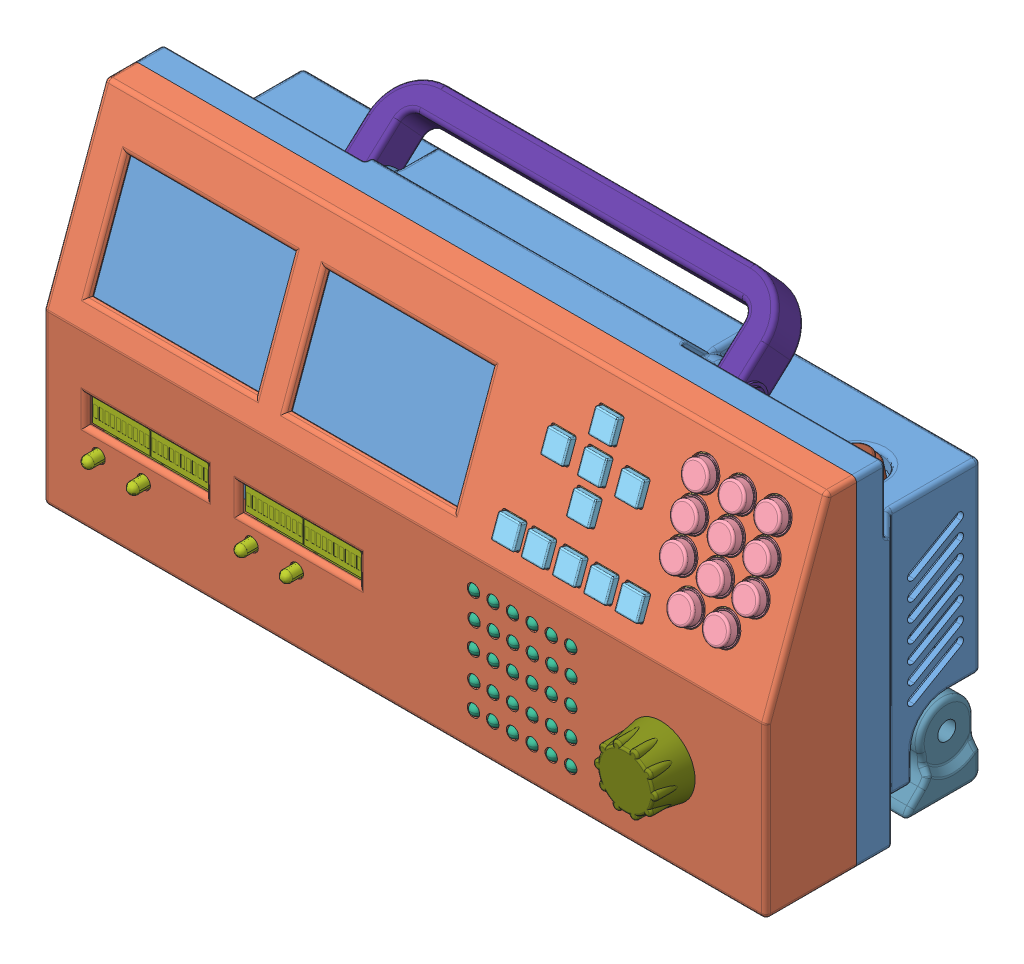
SolidWorks assembly Assembly, configuration Default. Lengths in mm.
Overall size (320 163.77 122.5).
42 component instances, 19 part files, 60 mates.
Components (placement in the parent):
- back_panel-1: back_panel [Default] at (2.4805 137.3007 327.5221) size (320 150.18 65)
- front_panel-1: front_panel [Default] at (322.4805 137.3007 342.5221) x (-1 0 0) z (0 0 -1) size (320 150.18 40)
- keypad_with_keycaps-1: keypad_with_keycaps [Default] at origin size (121.92 70.52 35.06)
  - Keypad-1: Keypad [Default] at (155.1031 162.0529 392.6379) x (1 0 0) z (0 0.34202 0.939693) size (121.92 71.12 10.8)
  - button_cap_round-1: button_cap_round [Default] at (304.9631 270.5 353.4325) x (-1 0 0) z (0 0.34202 0.939693) size (12.8 12.8 8.2)
  - button_cap_round-2: button_cap_round [Default] at (289.2151 270.5 353.4325) x (-1 0 0) z (0 0.34202 0.939693) size (12.8 12.8 8.2)
  - button_cap_round-3: button_cap_round [Default] at (272.9591 270.5 353.4325) x (-1 0 0) z (0 0.34202 0.939693) size (12.8 12.8 8.2)
  - button_cap_round-4: button_cap_round [Default] at (304.9631 257.1338 358.2973) x (-1 0 0) z (0 0.34202 0.939693) size (12.8 12.8 8.2)
  - button_cap_round-5: button_cap_round [Default] at (289.2151 257.1338 358.2973) x (-1 0 0) z (0 0.34202 0.939693) size (12.8 12.8 8.2)
  - button_cap_round-6: button_cap_round [Default] at (272.9591 257.1338 358.2973) x (-1 0 0) z (0 0.34202 0.939693) size (12.8 12.8 8.2)
  - button_cap_round-7: button_cap_round [Default] at (304.9631 243.7676 363.1622) x (-1 0 0) z (0 0.34202 0.939693) size (12.8 12.8 8.2)
  - button_cap_round-8: button_cap_round [Default] at (289.2151 243.7676 363.1622) x (-1 0 0) z (0 0.34202 0.939693) size (12.8 12.8 8.2)
  - button_cap_round-9: button_cap_round [Default] at (272.9591 243.7676 363.1622) x (-1 0 0) z (0 0.34202 0.939693) size (12.8 12.8 8.2)
  - button_cap_round-10: button_cap_round [Default] at (296.8351 230.4014 368.0271) x (-1 0 0) z (0 0.34202 0.939693) size (12.8 12.8 8.2)
  - button_cap_round-11: button_cap_round [Default] at (281.0871 230.4014 368.0271) x (-1 0 0) z (0 0.34202 0.939693) size (12.8 12.8 8.2)
  - button_cap_square-1: button_cap_square [Default] at (231.3031 255.2243 358.9923) x (1 0 0) z (0 0.34202 0.939693) size (10 10 6.2)
  - button_cap_square-2: button_cap_square [Default] at (231.3031 268.5905 354.1274) x (1 0 0) z (0 0.34202 0.939693) size (10 10 6.2)
  - button_cap_square-3: button_cap_square [Default] at (247.7131 255.2619 358.9787) x (1 0 0) z (0 0.34202 0.939693) size (10 10 6.2)
  - button_cap_square-4: button_cap_square [Default] at (215.0471 255.2243 358.9923) x (1 0 0) z (0 0.34202 0.939693) size (10 10 6.2)
  - button_cap_square-5: button_cap_square [Default] at (231.3031 241.9258 363.8326) x (1 0 0) z (0 0.34202 0.939693) size (10 10 6.2)
  - button_cap_square-6: button_cap_square [Default] at (204.8871 223.241 370.6333) x (1 0 0) z (0 0.34202 0.939693) size (10 10 6.2)
  - button_cap_square-7: button_cap_square [Default] at (218.0951 223.1216 370.6768) x (1 0 0) z (0 0.34202 0.939693) size (10 10 6.2)
  - button_cap_square-8: button_cap_square [Default] at (231.9381 223.1216 370.6768) x (1 0 0) z (0 0.34202 0.939693) size (10 10 6.2)
  - button_cap_square-9: button_cap_square [Default] at (245.7811 223.1216 370.6768) x (1 0 0) z (0 0.34202 0.939693) size (10 10 6.2)
  - button_cap_square-10: button_cap_square [Default] at (259.6241 223.1216 370.6768) x (1 0 0) z (0 0.34202 0.939693) size (10 10 6.2)
- LEDmatrix-1: LEDmatrix [Default] at (63.8045 79.9307 374.1221) size (64.13 65.66 10.01)
- LED_bars-1: LED_bars [Default] at (146.3805 197.4507 373.7106) x (0 -1 0) z (0 0 -1) size (39.75 57.75 38.1)
- LED_bars-2: LED_bars [Default] at (78.6305 197.4507 373.7106) x (0 -1 0) z (0 0 -1) size (39.75 57.75 38.1)
- potentiometer_B10K-1: potentiometer_B10K [Default] at (277.4318 177.2007 371.1221) x (0 -1 0) z (0 0 1) size (17 26.43 27.6)
- PSU-1: PSU [Default] at (165.6805 292.9007 291.6135) x (0 -1 0) z (0 0 1) size (46.8 37.5 15.1)
- MCU-2: MCU [Default] at (160.3185 237.8214 291.5693) x (-1 0 0) z (0 0 1) size (75.96 70.87 10.4)
- power switch-1: power switch [Default] at (287.4805 251.9761 307.5221) x (0.939025 0 0.34385) z (-0.34385 0 0.939025) size (19 38 19)
- DC_JACK-1: DC_JACK [Default] at (296.4805 202.3007 279.9221) x (0 1 0) z (0 0 -1) size (9.26 14.51 14.45)
- foot_right-1: foot_right [Default] at (27.4805 137.3007 327.5221) x (0 0 1) z (-1 0 0) size (32.66 35 18.16)
- foot_left-1: foot_left [Default] at (297.4805 137.3007 327.5221) x (0 0 1) z (-1 0 0) size (32.66 35 18.16)
- foot_chip-1: foot_chip [Default] at (25.0805 137.3007 342.5221) x (0 0 1) z (-1 0 0) size (23.38 5.24 35.8)
- foot_chip-2: foot_chip [Default] at (264.0805 137.3007 342.5221) x (0 0 1) z (-1 0 0) size (23.38 5.24 35.8)
- knob-1: knob [Default] at (277.4318 177.2007 383.9221) x (0 1 0) z (1 0 0) size (30 16.1 30)
- handle-1: handle [Default] at (162.4805 286.3387 299.3291) x (-1 0 0) z (0 0.673665 -0.739037) size (179 18 49)
- display_fastener_chip-1: display_fastener_chip [Default] at (102.4805 272.9078 350.6725) x (1 0 0) z (0 -0.939693 0.34202) size (35 1.6 17.5)
- LCD_display-1: LCD_display [Default] at (55.4805 244.1549 366.2457) x (1 0 0) z (0 -0.939693 0.34202) size (86 5 56)
- LCD_display-2: LCD_display [Default] at (143.4805 244.1549 366.2457) x (1 0 0) z (0 -0.939693 0.34202) size (86 5 56)
Mates (geometry in assembly coordinates):
- Coincident15: coincident aligned: plane of LED_bars-1 through (124.0204 187.2607 372.4121) normal (0 1 0); plane of LED_bars-2 through (56.2704 187.2607 372.4121) normal (0 1 0)
- Coincident16: coincident aligned: plane of LED_bars-1 through (124.0204 182.1807 380.4121) normal (0 0 1); plane of LED_bars-2 through (56.2704 182.1807 380.4121) normal (0 0 1)
- Distance3: distance = 6 mm anti-aligned: plane of front_panel-1 through (2.4805 137.3007 380.1221) normal (0 0 -1); plane of LEDmatrix-1 through (208.013 177.5302 374.1221) normal (0 0 1)
- Distance4: distance = 2 mm anti-aligned: plane of potentiometer_B10K-1 through (277.4318 177.2007 378.1221) normal (0 0 1); plane of front_panel-1 through (2.4805 137.3007 380.1221) normal (0 0 -1)
- Distance5: distance = 80 mm anti-aligned: plane of LEDmatrix-1 through (240.0805 144.7007 373.7106) normal (1 0 0); plane of front_panel-1 through (320.0805 137.3007 342.5221) normal (-1 0 0)
- Distance8: distance = 5 mm anti-aligned: plane of LEDmatrix-1 through (175.9455 144.7007 373.7106) normal (0 -1 0); plane of front_panel-1 through (2.4805 139.7007 342.5221) normal (0 1 0)
- Distance9: distance = 16 mm anti-aligned: plane of LED_bars-2 through (20.8805 197.4507 374.1221) normal (-1 0 0); plane of front_panel-1 through (4.8805 137.3007 342.5221) normal (1 0 0)
- Distance10: distance = 10 mm anti-aligned: plane of LED_bars-2 through (78.6305 157.7007 374.1221) normal (1 0 0); plane of LED_bars-1 through (88.6305 197.4507 374.1221) normal (-1 0 0)
- Distance11: distance = 6 mm anti-aligned: plane of LED_bars-2 through (49.7555 177.5757 374.1221) normal (0 0 1); plane of front_panel-1 through (2.4805 137.3007 380.1221) normal (0 0 -1)
- Distance13: distance = 18 mm anti-aligned: plane of front_panel-1 through (2.4805 139.7007 342.5221) normal (0 1 0); plane of LED_bars-1 through (88.6305 157.7007 374.1221) normal (0 -1 0)
- Coincident31: coincident aligned: plane of back_panel-1 through (322.4805 137.3007 342.5221) normal (1 0 0); plane of front_panel-1 through (322.4805 137.3007 342.5221) normal (1 0 0)
- Coincident32: coincident aligned: plane of back_panel-1 through (2.4805 287.4761 342.5221) normal (0 1 0); plane of front_panel-1 through (2.4805 287.4761 355.1605) normal (0 1 0)
- Coincident33: coincident anti-aligned: plane of back_panel-1 through (2.4805 137.3007 342.5221) normal (0 0 1); plane of front_panel-1 through (2.4805 287.4761 342.5221) normal (0 0 -1)
- Distance17: distance = 70 mm anti-aligned: plane of MCU-2 through (84.8805 168.2254 289.9221) normal (-1 0 0); plane of back_panel-1 through (14.8805 277.4761 277.5221) normal (1 0 0)
- Width2: width anti-aligned: plane of MCU-2 through (86.1505 237.8214 289.9221) normal (0 1 0); plane of back_panel-1 through (159.0485 166.9554 289.9221) normal (0 -1 0); plane of MCU-2 through (322.4805 255.0761 330.0221) normal (0 -1 0); plane of back_panel-1 through (312.4805 149.7007 277.5221) normal (0 1 0)
- Distance18: distance = 70 mm aligned: plane of PSU-1 through (240.0805 200.4307 289.9221) normal (-1 0 0); plane of back_panel-1 through (310.0805 277.4761 277.5221) normal (-1 0 0)
- Distance19: distance = 5.2 mm anti-aligned: plane of PSU-1 through (241.3505 154.9007 289.9221) normal (0 -1 0); plane of back_panel-1 through (312.4805 149.7007 277.5221) normal (0 1 0)
- Coincident37: coincident anti-aligned: plane of back_panel-1 through (88.2285 169.9054 289.9221) normal (0 0 1); plane of MCU-2 through (122.5995 202.3884 289.9221) normal (0 0 -1)
- Coincident38: coincident anti-aligned: plane of back_panel-1 through (243.1805 198.6507 289.9221) normal (0 0 1); plane of PSU-1 through (258.8305 178.3007 289.9221) normal (0 0 -1)
- Concentric2: concentric aligned: cylinder of back_panel-1 through (287.4805 230.1913 307.5221) axis (0 1 0) radius 6.5; cylinder of power switch-1 through (287.4805 223.9761 307.5221) axis (0 1 0) radius 5.25
- Distance14: distance = 1 mm anti-aligned: plane of power switch-1 through (287.4805 251.9761 307.5221) normal (0 -1 0); plane of back_panel-1 through (287.4805 250.9761 307.5221) normal (0 1 0)
- Parallel1: parallel aligned: plane of back_panel-1 through (310.0805 277.4761 277.5221) normal (-1 0 0); plane of DC_JACK-1 through (290.9805 206.5507 279.9221) normal (-1 0 0)
- Concentric4: concentric anti-aligned: circle of DC_JACK-1; cylinder of back_panel-1 through (297.4805 202.3007 298.3069) axis (0 0 -1) radius 6.5
- Coincident42: coincident anti-aligned: plane of back_panel-1 through (2.4805 137.3007 279.9221) normal (0 0 1); plane of DC_JACK-1 through (296.4805 202.3007 279.9221) normal (0 0 -1)
- Parallel2: parallel aligned: plane of front_panel-1 through (320.0805 137.3007 342.5221) normal (-1 0 0); plane of potentiometer_B10K-1 through (265.0805 184.7007 378.1221) normal (-1 0 0)
- Distance15: distance = 55 mm aligned: plane of potentiometer_B10K-1 through (265.0805 184.7007 378.1221) normal (-1 0 0); plane of front_panel-1 through (320.0805 137.3007 342.5221) normal (-1 0 0)
- Distance16: distance = 30 mm anti-aligned: plane of potentiometer_B10K-1 through (265.0805 169.7007 378.1221) normal (0 -1 0); plane of front_panel-1 through (2.4805 139.7007 342.5221) normal (0 1 0)
- InPlace1: in place: plane of back_panel-1 through (27.4805 160.3007 292.5221) normal (-1 0 0); plane of ? through (27.4805 0 0) normal (-1 0 0); moOrthogonalPlaneRef_w of back_panel-1 through (27.4805 160.3007 292.5221) normal (-1 0 0); plane of ? through (27.4805 0 0) normal (0 1 0); plane of back_panel-1 through (27.4805 160.3007 292.5221) normal (-1 0 0); plane of ? through (27.4805 0 0) normal (0 0 1); plane of back_panel-1 through (27.4805 160.3007 292.5221) normal (-1 0 0); unknown of foot_right-1
- Coincident43: coincident aligned: plane of back_panel-1; plane of foot_right-1
- Coincident44: coincident aligned: moOrthogonalPlaneRef_w of back_panel-1 through (27.4805 137.3007 327.5221) normal (0 1 0); plane of footer^Assembly-1 through (27.4805 137.3007 327.5221) normal (0 1 0)
- Coincident45: coincident anti-aligned: moOrthogonalPlaneRef_w of back_panel-1 through (27.4805 137.3007 327.5221) normal (0 0 -1); plane of footer^Assembly-1 through (27.4805 137.3007 327.5221) normal (0 0 1)
- Coincident43: coincident anti-aligned: plane of back_panel-1 through (297.4805 160.3007 292.5221) normal (1 0 0); plane of foot_left-1 through (297.4805 137.3007 307.0196) normal (-1 0 0)
- Concentric5: concentric aligned: circle of foot_right-1; circle of foot_left-1
- InPlace2: in place: plane of front_panel-1 through (25.0805 141.3007 342.5221) normal (-1 0 0); plane of ? through (25.0805 0 0) normal (-1 0 0); plane of front_panel-1 through (25.0805 141.3007 342.5221) normal (-1 0 0); plane of ? through (25.0805 0 0) normal (0 1 0); plane of front_panel-1 through (25.0805 141.3007 342.5221) normal (-1 0 0); plane of ? through (25.0805 0 0) normal (0 0 1); plane of front_panel-1 through (25.0805 141.3007 342.5221) normal (-1 0 0); unknown of foot_chip-1
- Coincident46: coincident aligned: plane of front_panel-1; plane of foot_chip-1
- Coincident47: coincident aligned: moOrthogonalPlaneRef_w of front_panel-1 through (25.0805 137.3007 342.5221) normal (0 1 0); plane of foot_chip-1 through (25.0805 137.3007 342.5221) normal (0 1 0)
- Coincident48: coincident anti-aligned: moOrthogonalPlaneRef_w of front_panel-1 through (25.0805 137.3007 342.5221) normal (0 0 -1); plane of foot_chip-1 through (25.0805 137.3007 342.5221) normal (0 0 1)
- Coincident49: coincident aligned: plane of front_panel-1 through (299.8805 141.3007 342.5221) normal (1 0 0); plane of foot_chip-2 through (299.8805 141.3007 342.5221) normal (1 0 0)
- Concentric6: concentric aligned: cylinder of front_panel-1 through (304.0524 141.3007 369.0221) axis (-1 0 0) radius 1.475; cylinder of foot_chip-2 through (303.3736 141.3007 369.0221) axis (-1 0 0) radius 1.235
- Coincident50: coincident aligned: plane of foot_right-1 through (9.4805 137.3007 280.5221) normal (0 -1 0); plane of foot_left-1 through (315.4805 137.3007 280.5221) normal (0 -1 0)
- Coincident51: coincident aligned: plane of foot_chip-1 through (1.3719 137.3007 346.5777) normal (0 -1 0); plane of foot_chip-2 through (240.3719 137.3007 346.5777) normal (0 -1 0)
- Concentric8: concentric anti-aligned: cylinder of potentiometer_B10K-1 through (277.4318 177.2007 387.7221) axis (0 0 -1) radius 3.5; cylinder of knob-1 through (277.4318 177.2007 371.477) axis (0 0 1) radius 4.4
- Coincident52: coincident anti-aligned: plane of potentiometer_B10K-1 through (277.4318 177.2007 398.7221) normal (0 0 1); plane of knob-1 through (277.4318 177.2007 398.7221) normal (0 0 -1)
- Width4: width aligned: plane of handle-1 through (85.9805 315.6476 280.5358) normal (1 0 0); plane of handle-1 through (238.9805 315.6476 280.5358) normal (-1 0 0); plane of back_panel-1 through (238.4805 267.4761 320.0221) normal (1 0 0); plane of back_panel-1 through (86.4805 267.4761 320.0221) normal (-1 0 0)
- Concentric11: concentric aligned: circle of back_panel-1; circle of handle-1
- Coincident53: coincident anti-aligned: plane of front_panel-1 through (322.4805 156.3304 394.8059) normal (0 -0.34202 -0.939693); plane of display_fastener_chip-1 through (102.4805 273.455 352.176) normal (0 0.34202 0.939693)
- Concentric12: concentric anti-aligned: circle of front_panel-1; circle of display_fastener_chip-1
- LimitAngle1: limit planar angle = 0.739157 rad aligned: plane of back_panel-1 through (322.4805 257.4761 330.0221) normal (0 1 0); plane of handle-1 through (85.9805 301.074 296.5236) normal (0 0.739037 0.673665)
- LimitAngle2: limit planar angle = 0 rad aligned: plane of front_panel-1 through (322.4805 137.3007 342.5221) normal (0 1 0); plane of knob-1 through (277.4318 177.2007 383.9221) normal (0 1 0)
- Concentric13: concentric aligned: circle of front_panel-1; cylinder of knob-1 through (277.4318 177.2007 371.077) axis (0 0 1) radius 2.8
- Distance20: distance = 1 mm anti-aligned: plane of knob-1 through (277.4318 177.2007 383.9221) normal (0 0 -1); plane of front_panel-1 through (2.4805 137.3007 382.5221) normal (0 0 1)
- Coincident124: coincident anti-aligned: plane of front_panel-1 through (2.4805 211.4798 380.2668) normal (0 -0.34202 -0.939693); plane of LCD_display-1 through (55.4805 244.8389 368.1251) normal (0 0.34202 0.939693)
- Width5: width aligned: plane of front_panel-1 through (17.4805 221.6976 379.1019) normal (0.866025 0.17101 0.469846); plane of front_panel-1 through (93.4805 221.6976 379.1019) normal (-0.866025 0.17101 0.469846); plane of LCD_display-1 through (18.4805 221.8164 376.5046) normal (-1 0 0); plane of LCD_display-1 through (92.4805 221.8164 376.5046) normal (1 0 0)
- Width6: width aligned: plane of front_panel-1 through (17.4805 269.6219 361.6589) normal (0 -0.642788 0.766044); plane of front_panel-1 through (17.4805 221.6976 379.1019) normal (0 0.984808 0.173648); plane of LCD_display-1 through (18.4805 267.8614 359.7456) normal (0 0.939693 -0.34202); plane of LCD_display-1 through (18.4805 221.8164 376.5046) normal (0 -0.939693 0.34202)
- Coincident125: coincident anti-aligned: plane of front_panel-1 through (2.4805 211.4798 380.2668) normal (0 -0.34202 -0.939693); plane of LCD_display-2 through (143.4805 244.8389 368.1251) normal (0 0.34202 0.939693)
- Width7: width aligned: plane of front_panel-1 through (17.4805 269.6219 361.6589) normal (0 -0.642788 0.766044); plane of front_panel-1 through (17.4805 221.6976 379.1019) normal (0 0.984808 0.173648); plane of LCD_display-2 through (106.4805 267.8614 359.7456) normal (0 0.939693 -0.34202); plane of LCD_display-2 through (106.4805 221.8164 376.5046) normal (0 -0.939693 0.34202)
- Width8: width aligned: plane of front_panel-1 through (105.4805 221.6976 379.1019) normal (0.866025 0.17101 0.469846); plane of front_panel-1 through (181.4805 221.6976 379.1019) normal (-0.866025 0.17101 0.469846); plane of LCD_display-2 through (106.4805 221.8164 376.5046) normal (-1 0 0); plane of LCD_display-2 through (180.4805 221.8164 376.5046) normal (1 0 0)
- Width9: width aligned: plane of Assem1^Assembly-1/Keypad-1 through (195.7431 212.7514 373.7473) normal (-1 0 0); plane of Assem1^Assembly-1/Keypad-1 through (317.6631 277.1955 350.2915) normal (1 0 0); plane of front_panel-1 through (320.0805 137.3007 342.5221) normal (-1 0 0); plane of front_panel-1 through (193.3258 271.5577 349.8869) normal (1 0 0)
- Distance21: distance = 2 mm aligned: plane of Assem1^Assembly-1/Keypad-1 through (316.3931 211.558 374.1817) normal (0 -0.939693 0.34202); plane of front_panel-1 through (193.3258 212.6478 371.3283) normal (0 -0.939693 0.34202)
- Coincident126: coincident anti-aligned: plane of front_panel-1 through (198.2831 276.1428 351.1126) normal (0 -0.34202 -0.939693); plane of Assem1^Assembly-1/Keypad-1 through (256.6851 245.1241 362.4025) normal (0 0.34202 0.939693)
